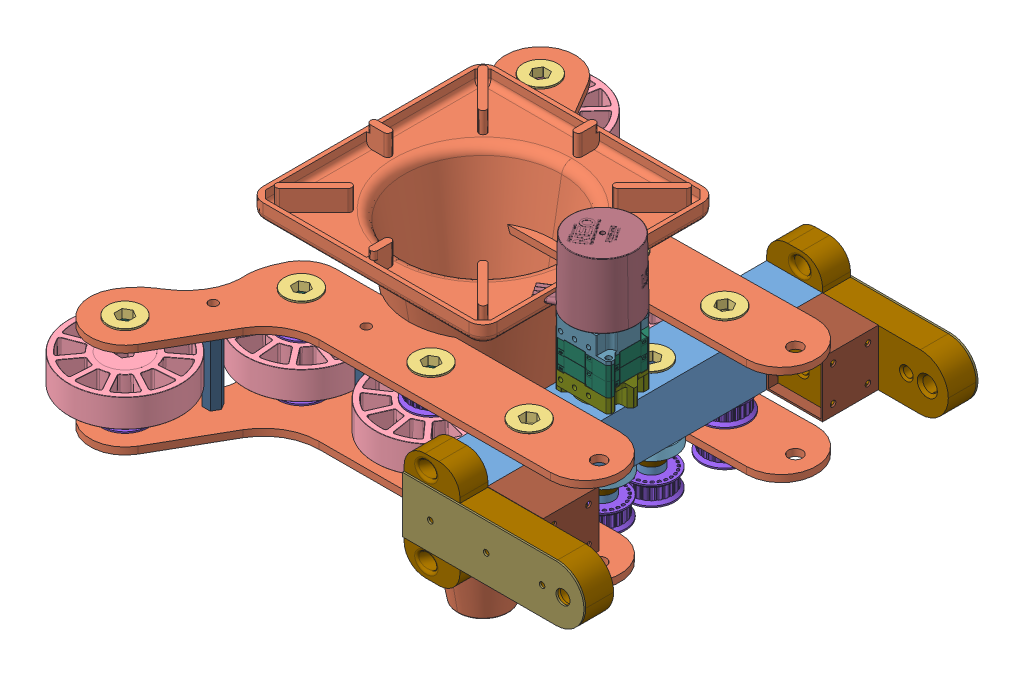
SolidWorks assembly Intake_Claw_2.0, configuration Default. Lengths in mm.
Overall size (474.27 365.54 510.07).
111 component instances, 20 part files, 307 mates.
Components (placement in the parent):
- Claw_Crossbar-1: Claw_Crossbar [Default] at origin size (50.8 50.8 304.8)
- Claw_Intake_Plate_3_Wheel-3: Claw_Intake_Plate_3_Wheel [Default] at (-63.4996 52.3773 241.5528) x (-0.002844 0 -0.999996) z (0.999996 0 -0.002844) size (165.24 6.35 379.41)
- am-2986 FR8ZZ Hex Bearing.step-1: am-2986 FR8ZZ Hex Bearing.step [Default] at (25.4 44.3967 241.3) x (-0.023449 0 -0.999725) z (0 1 0) size (31.12 31.12 7.93)
- am-2986 FR8ZZ Hex Bearing.step-3: am-2986 FR8ZZ Hex Bearing.step [Default] at (-239.4221 52.324 343.7898) x (0 0 -1) z (0 1 0) size (31.12 31.12 7.93)
- am-2986 FR8ZZ Hex Bearing.step-5: am-2986 FR8ZZ Hex Bearing.step [Default] at (25.4 52.324 241.3) x (0 0 -1) z (0 1 0) size (31.12 31.12 7.93)
- am-2986 FR8ZZ Hex Bearing.step-11: am-2986 FR8ZZ Hex Bearing.step [Default] at (-63.4996 52.324 241.5528) x (0 0 -1) z (0 1 0) size (31.12 31.12 7.93)
- am-2986 FR8ZZ Hex Bearing.step-12: am-2986 FR8ZZ Hex Bearing.step [Default] at (-180.9742 52.324 241.8869) x (0 0 -1) z (0 1 0) size (31.12 31.12 7.93)
- Intake_Plate_Assembly-1: Intake_Plate_Assembly [Default] at (-25.3851 110.6877 261.8842) x (0.99204 0 0.125922) z (0.125922 0 -0.99204)
- Intake_Plate_Assembly_2-1: Intake_Plate_Assembly_2 [Default] at (-16.4979 -120.1924 40.8533) x (0.996656 0 -0.081713) z (0.081713 0 0.996656)
- Intake_Plate_Assembly_2-2: Intake_Plate_Assembly_2 [Default] at (-25.364 170.9924 261.8868) x (0.99204 0 0.125922) z (0.125922 0 -0.99204)
- am-3480 4IN 500Hex Bore Compliant Wheel REV2.STEP-1: am-3480 4IN 500Hex Bore Compliant Wheel REV2.STEP [Default] at (-227.1156 24.621 332.519) x (0.873407 0 -0.486991) z (0 -1 0) size (101.6 101.6 25.4)
- am-3480 4IN 500Hex Bore Compliant Wheel REV2.STEP-2: am-3480 4IN 500Hex Bore Compliant Wheel REV2.STEP [Default] at (-170.4614 24.621 228.9267) x (0.792175 0 -0.610293) z (0 -1 0) size (101.6 101.6 25.4)
- am-3480 4IN 500Hex Bore Compliant Wheel REV2.STEP-3: am-3480 4IN 500Hex Bore Compliant Wheel REV2.STEP [Default] at (-68.8044 24.621 257.3751) x (-0.528092 0 0.849187) z (0 -1 0) size (101.6 101.6 25.4)
- am-3480 4IN 500Hex Bore Compliant Wheel REV2.STEP-4: am-3480 4IN 500Hex Bore Compliant Wheel REV2.STEP [Default] at (-47.059 24.621 61.63) x (0.998282 0 0.058584) z (0 -1 0) size (101.6 101.6 25.4)
- am-3480 4IN 500Hex Bore Compliant Wheel REV2.STEP-5: am-3480 4IN 500Hex Bore Compliant Wheel REV2.STEP [Default] at (-164.7239 24.621 62.024) x (1 0 0) z (0 -1 0) size (101.6 101.6 25.4)
- am-3480 4IN 500Hex Bore Compliant Wheel REV2.STEP-6: am-3480 4IN 500Hex Bore Compliant Wheel REV2.STEP [Default] at (-248.6981 24.621 -49.9144) x (-0.252916 0 -0.967488) z (0 -1 0) size (101.6 101.6 25.4)
- am-2986 FR8ZZ Hex Bearing.step-13: am-2986 FR8ZZ Hex Bearing.step [Default] at (25.4 6.4033 130.175) x (-0.368447 0 0.929649) z (0 -1 0) size (31.12 31.12 7.93)
- am-2986 FR8ZZ Hex Bearing.step-14: am-2986 FR8ZZ Hex Bearing.step [Default] at (25.4 44.3967 130.175) x (-0.368447 0 0.929649) z (0 1 0) size (31.12 31.12 7.93)
- Claw_Drive_Gear-1: Claw_Drive_Gear [Default] at (25.4 -14.1478 130.175) x (0.993752 0 0.111608) z (-0.111608 0 0.993752) size (43.69 9.45 43.69)
- Claw_Drive_Gear-2: Claw_Drive_Gear [Default] at (25.4 -14.1478 174.625) x (0.964298 0 0.26482) z (-0.26482 0 0.964298) size (43.69 9.45 43.69)
- half_inch_hex_spacer_0.125inch-1: half_inch_hex_spacer_0.125inch [Default] at (25.4 -4.699 130.175) x (0.999916 0 -0.012929) z (0.012929 0 0.999916) size (20.32 3.17 20.32)
- half_inch_hex_spacer_0.125inch-2: half_inch_hex_spacer_0.125inch [Default] at (25.4 -4.699 174.625) x (0.980488 0 0.196577) z (-0.196577 0 0.980488) size (20.32 3.17 20.32)
- am-2986 FR8ZZ Hex Bearing.step-16: am-2986 FR8ZZ Hex Bearing.step [Default] at (25.4 44.3967 63.5) x (-0.023449 0 -0.999725) z (0 1 0) size (31.12 31.12 7.93)
- am-2986 FR8ZZ Hex Bearing.step-18: am-2986 FR8ZZ Hex Bearing.step [Default] at (25.4 6.4033 63.5) x (-0.368447 0 0.929649) z (0 -1 0) size (31.12 31.12 7.93)
- am-2986 FR8ZZ Hex Bearing.step-19: am-2986 FR8ZZ Hex Bearing.step [Default] at (25.4 6.4033 241.3) x (-0.368447 0 0.929649) z (0 -1 0) size (31.12 31.12 7.93)
- half_inch_hex_spacer_0.1875inch-1: half_inch_hex_spacer_0.1875inch [Default] at (25.4 52.324 63.5) size (20.32 4.76 20.32)
- 24_tooth_5mmHTD_timing_belt_pulley_9mm-3: 24_tooth_5mmHTD_timing_belt_pulley_9mm [Default] at (-180.9742 35.179 241.8869) x (0.987086 0 0.160191) z (0 -1 0) size (42.16 42.16 17.78)
- 24_tooth_5mmHTD_timing_belt_pulley_9mm-8: 24_tooth_5mmHTD_timing_belt_pulley_9mm [Default] at (25.4 -47.1678 174.625) x (0.071014 0 0.997475) z (0 -1 0) size (42.16 42.16 17.78)
- 24_tooth_5mmHTD_timing_belt_pulley_9mm-9: 24_tooth_5mmHTD_timing_belt_pulley_9mm [Default] at (25.4 -47.1678 130.175) x (0.476247 0 -0.879312) z (0 -1 0) size (42.16 42.16 17.78)
- 24_tooth_5mmHTD_timing_belt_pulley_9mm-13: 24_tooth_5mmHTD_timing_belt_pulley_9mm [Default] at (-180.9613 35.179 65.8749) x (0.911482 0 -0.411341) z (0 -1 0) size (42.16 42.16 17.78)
- 24_tooth_5mmHTD_timing_belt_pulley_9mm-15: 24_tooth_5mmHTD_timing_belt_pulley_9mm [Default] at (-63.4996 35.179 241.5528) x (0.911482 0 -0.411341) z (0 -1 0) size (42.16 42.16 17.78)
- 24_tooth_5mmHTD_timing_belt_pulley_9mm-16: 24_tooth_5mmHTD_timing_belt_pulley_9mm [Default] at (-63.4941 35.179 64.523) x (0.84545 0 -0.534054) z (0 -1 0) size (42.16 42.16 17.78)
- half_inch_hex_spacer_0.125inch-13: half_inch_hex_spacer_0.125inch [Default] at (-63.4941 2.794 64.523) size (20.32 3.17 20.32)
- half_inch_hex_spacer_0.125inch-14: half_inch_hex_spacer_0.125inch [Default] at (-180.9613 2.794 65.8749) size (20.32 3.17 20.32)
- half_inch_hex_spacer_0.125inch-15: half_inch_hex_spacer_0.125inch [Default] at (-240.8657 2.794 -35.1788) size (20.32 3.17 20.32)
- half_inch_hex_spacer_0.125inch-16: half_inch_hex_spacer_0.125inch [Default] at (-63.4996 2.794 241.5528) size (20.32 3.17 20.32)
- half_inch_hex_spacer_0.125inch-17: half_inch_hex_spacer_0.125inch [Default] at (-180.9742 2.794 241.8869) size (20.32 3.17 20.32)
- half_inch_hex_spacer_0.125inch-18: half_inch_hex_spacer_0.125inch [Default] at (-239.4221 2.794 343.7898) size (20.32 3.17 20.32)
- Grabber_Spring_Mount-1: Grabber_Spring_Mount [Default] at (49.2125 48.5775 260.35) x (-1 0 0) z (0 0 1) size (165.1 97.79 69.85)
- Grabber_Spring_Mount-2: Grabber_Spring_Mount [Default] at (48.5775 1.5875 44.45) x (-1 0 0) z (0 0 -1) size (165.1 97.79 69.85)
- 24_tooth_5mmHTD_timing_belt_pulley_9mm-17: 24_tooth_5mmHTD_timing_belt_pulley_9mm [Default] at (25.4 -18.669 241.3) x (0.782455 0 -0.622708) z (0 -1 0) size (42.16 42.16 17.78)
- 24_tooth_5mmHTD_timing_belt_pulley_9mm-18: 24_tooth_5mmHTD_timing_belt_pulley_9mm [Default] at (25.4 -18.669 63.5) x (0.782455 0 -0.622708) z (0 -1 0) size (42.16 42.16 17.78)
- half_inch_hex_spacer_0.125inch-19: half_inch_hex_spacer_0.125inch [Default] at (25.4 -4.699 63.5) size (20.32 3.17 20.32)
- half_inch_hex_spacer_0.125inch-20: half_inch_hex_spacer_0.125inch [Default] at (25.4 -4.699 241.3) size (20.32 3.17 20.32)
- half_inch_hex_spacer_0.125inch-21: half_inch_hex_spacer_0.125inch [Default] at (-63.4941 -0.381 64.523) size (20.32 3.17 20.32)
- half_inch_hex_spacer_0.125inch-22: half_inch_hex_spacer_0.125inch [Default] at (-180.9613 -0.381 65.8749) size (20.32 3.17 20.32)
- half_inch_hex_spacer_0.125inch-23: half_inch_hex_spacer_0.125inch [Default] at (-240.8657 -0.381 -35.1788) size (20.32 3.17 20.32)
- half_inch_hex_spacer_0.125inch-24: half_inch_hex_spacer_0.125inch [Default] at (-239.4221 -0.381 343.7898) size (20.32 3.17 20.32)
- half_inch_hex_spacer_0.125inch-25: half_inch_hex_spacer_0.125inch [Default] at (-180.9742 -0.381 241.8869) size (20.32 3.17 20.32)
- half_inch_hex_spacer_0.125inch-26: half_inch_hex_spacer_0.125inch [Default] at (-63.4996 -0.381 241.5528) size (20.32 3.17 20.32)
- half_inch_hex_spacer_0.125inch-27: half_inch_hex_spacer_0.125inch [Default] at (-63.4996 -21.336 241.5528) size (20.32 3.17 20.32)
- half_inch_hex_spacer_0.125inch-28: half_inch_hex_spacer_0.125inch [Default] at (-180.9742 -21.336 241.8869) size (20.32 3.17 20.32)
- half_inch_hex_spacer_0.125inch-29: half_inch_hex_spacer_0.125inch [Default] at (-239.4221 -21.336 343.7898) size (20.32 3.17 20.32)
- half_inch_hex_spacer_0.125inch-30: half_inch_hex_spacer_0.125inch [Default] at (-63.4941 -21.336 64.523) size (20.32 3.17 20.32)
- half_inch_hex_spacer_0.125inch-31: half_inch_hex_spacer_0.125inch [Default] at (-180.9613 -21.336 65.8749) size (20.32 3.17 20.32)
- half_inch_hex_spacer_0.125inch-32: half_inch_hex_spacer_0.125inch [Default] at (-240.8657 -21.336 -35.1788) size (20.32 3.17 20.32)
- 24_tooth_5mmHTD_timing_belt_pulley_9mm-19: 24_tooth_5mmHTD_timing_belt_pulley_9mm [Default] at (-63.4941 -14.351 64.523) x (1 0 0) z (0 -1 0) size (42.16 42.16 17.78)
- 24_tooth_5mmHTD_timing_belt_pulley_9mm-20: 24_tooth_5mmHTD_timing_belt_pulley_9mm [Default] at (-180.9613 -14.351 65.8749) x (1 0 0) z (0 -1 0) size (42.16 42.16 17.78)
- 24_tooth_5mmHTD_timing_belt_pulley_9mm-21: 24_tooth_5mmHTD_timing_belt_pulley_9mm [Default] at (-240.8657 -14.351 -35.1788) x (1 0 0) z (0 -1 0) size (42.16 42.16 17.78)
- 24_tooth_5mmHTD_timing_belt_pulley_9mm-22: 24_tooth_5mmHTD_timing_belt_pulley_9mm [Default] at (-239.4221 -14.351 343.7898) x (1 0 0) z (0 -1 0) size (42.16 42.16 17.78)
- 24_tooth_5mmHTD_timing_belt_pulley_9mm-23: 24_tooth_5mmHTD_timing_belt_pulley_9mm [Default] at (-180.9742 -14.351 241.8869) x (1 0 0) z (0 -1 0) size (42.16 42.16 17.78)
- 24_tooth_5mmHTD_timing_belt_pulley_9mm-24: 24_tooth_5mmHTD_timing_belt_pulley_9mm [Default] at (-63.4996 -14.351 241.5528) x (1 0 0) z (0 -1 0) size (42.16 42.16 17.78)
- half_inch_hex_spacer_0.125inch-33: half_inch_hex_spacer_0.125inch [Default] at (25.4 -25.654 63.5) size (20.32 3.17 20.32)
- half_inch_hex_spacer_0.125inch-34: half_inch_hex_spacer_0.125inch [Default] at (25.4 -25.654 241.3) size (20.32 3.17 20.32)
- Intake_Plate_Assembly-3: Intake_Plate_Assembly [Default] at (-25.3851 78.6304 261.8842) x (0.99204 0 0.125922) z (0.125922 0 -0.99204)
- Intake_Plate_Assembly_2-4: Intake_Plate_Assembly_2 [Default] at (-16.4979 -152.2498 40.8533) x (0.996656 0 -0.081713) z (0.081713 0 0.996656)
- grabber_stand_off-1: grabber_stand_off [Default] at (-122.2369 52.3977 241.7198) x (1 0 0) z (0 -1 0) size (14.66 12.7 76.2)
- grabber_stand_off-3: grabber_stand_off [Default] at (-210.1981 52.3773 292.8384) x (1 0 0) z (0 -1 0) size (14.66 12.7 76.2)
- grabber_stand_off-4: grabber_stand_off [Default] at (-210.9135 44.5398 15.3481) x (-0.606361 0 0.795189) z (0 -1 0) size (14.66 12.7 76.2)
- grabber_stand_off-5: grabber_stand_off [Default] at (-122.2277 50.6322 65.199) x (1 0 0) z (0 -1 0) size (14.66 12.7 76.2)
- Crossbar_Bracket-1: Crossbar_Bracket [Default] at (101.6 0 0) x (0 1 0) z (0 0 1) size (50.8 50.8 50.8)
- Crossbar_Bracket-2: Crossbar_Bracket [Default] at (101.6 0 254) x (0 1 0) z (0 0 1) size (50.8 50.8 50.8)
- Claw_Pivot_Plate-1: Claw_Pivot_Plate [Default] at (0.635 -0.3175 330.2) size (165.1 50.8 1.59)
- Claw_Pivot_Plate-2: Claw_Pivot_Plate [Default] at (0 -0.3175 -26.9875) size (165.1 50.8 1.59)
- half_inch_hex_spacer_0.125inch-35: half_inch_hex_spacer_0.125inch [Default] at (-63.4996 49.149 241.5528) size (20.32 3.17 20.32)
- half_inch_hex_spacer_0.125inch-36: half_inch_hex_spacer_0.125inch [Default] at (-180.9742 49.149 241.8869) size (20.32 3.17 20.32)
- half_inch_hex_spacer_0.125inch-37: half_inch_hex_spacer_0.125inch [Default] at (-239.4221 49.149 343.7898) size (20.32 3.17 20.32)
- half_inch_hex_spacer_0.125inch-38: half_inch_hex_spacer_0.125inch [Default] at (-63.4941 49.149 64.523) size (20.32 3.17 20.32)
- half_inch_hex_spacer_0.125inch-39: half_inch_hex_spacer_0.125inch [Default] at (-180.9613 49.149 65.8749) size (20.32 3.17 20.32)
- Claw_Intake_Plate_3_Wheel-4: Claw_Intake_Plate_3_Wheel [Default] at (-63.4996 -27.7393 241.5528) x (-0.002844 0 -0.999996) z (0.999996 0 -0.002844) size (165.24 6.35 379.41)
- Claw_Intake_Plate_3_Wheel-5: Claw_Intake_Plate_3_Wheel [Default] at (-63.4941 58.7273 64.523) x (0.011508 0 0.999934) z (0.999934 0 -0.011508) size (165.24 6.35 379.41)
- Claw_Intake_Plate_3_Wheel-6: Claw_Intake_Plate_3_Wheel [Default] at (-63.4941 -25.7073 64.523) x (0.011508 0 0.999934) z (0.999934 0 -0.011508) size (165.24 6.35 379.41)
- am-2986 FR8ZZ Hex Bearing.step-20: am-2986 FR8ZZ Hex Bearing.step [Default] at (25.4 -21.336 241.3) x (1 0 0) z (0 -1 0) size (31.12 31.12 7.93)
- am-2986 FR8ZZ Hex Bearing.step-21: am-2986 FR8ZZ Hex Bearing.step [Default] at (-63.4996 -21.336 241.5528) x (0.820291 0 -0.571946) z (0 -1 0) size (31.12 31.12 7.93)
- am-2986 FR8ZZ Hex Bearing.step-22: am-2986 FR8ZZ Hex Bearing.step [Default] at (-180.9742 -21.336 241.8869) x (1 0 0) z (0 -1 0) size (31.12 31.12 7.93)
- am-2986 FR8ZZ Hex Bearing.step-23: am-2986 FR8ZZ Hex Bearing.step [Default] at (-239.4221 -21.336 343.7898) x (1 0 0) z (0 -1 0) size (31.12 31.12 7.93)
- am-2986 FR8ZZ Hex Bearing.step-24: am-2986 FR8ZZ Hex Bearing.step [Default] at (25.4 -25.654 63.5) x (1 0 0) z (0 -1 0) size (31.12 31.12 7.93)
- am-2986 FR8ZZ Hex Bearing.step-25: am-2986 FR8ZZ Hex Bearing.step [Default] at (-63.4941 -25.654 64.523) x (1 0 0) z (0 -1 0) size (31.12 31.12 7.93)
- am-2986 FR8ZZ Hex Bearing.step-26: am-2986 FR8ZZ Hex Bearing.step [Default] at (-240.8657 -25.654 -35.1788) x (1 0 0) z (0 -1 0) size (31.12 31.12 7.93)
- am-2986 FR8ZZ Hex Bearing.step-27: am-2986 FR8ZZ Hex Bearing.step [Default] at (-180.9613 -25.654 65.8749) x (1 0 0) z (0 -1 0) size (31.12 31.12 7.93)
- am-2986 FR8ZZ Hex Bearing.step-28: am-2986 FR8ZZ Hex Bearing.step [Default] at (25.4 52.324 63.5) x (1 0 0) z (0 1 0) size (31.12 31.12 7.93)
- am-2986 FR8ZZ Hex Bearing.step-29: am-2986 FR8ZZ Hex Bearing.step [Default] at (-63.4941 52.324 64.523) x (1 0 0) z (0 1 0) size (31.12 31.12 7.93)
- am-2986 FR8ZZ Hex Bearing.step-30: am-2986 FR8ZZ Hex Bearing.step [Default] at (-180.9613 52.324 65.8749) x (1 0 0) z (0 1 0) size (31.12 31.12 7.93)
- am-2986 FR8ZZ Hex Bearing.step-31: am-2986 FR8ZZ Hex Bearing.step [Default] at (-240.8657 52.324 -35.1788) x (1 0 0) z (0 1 0) size (31.12 31.12 7.93)
- am-2986 FR8ZZ Hex Bearing.step-32: am-2986 FR8ZZ Hex Bearing.step [Default] at (25.4 6.4033 174.625) x (-0.500268 0 0.865871) z (0 -1 0) size (31.12 31.12 7.93)
- Neo_with_2_Stage_Gearbox-1: Neo_with_2_Stage_Gearbox [Default] at (26.2874 219.325 175.8085) x (0.980561 0 0.196216) z (0 -1 0) size (73.48 69 161.54)
  - REV-21-1650-V1.1.step-1: REV-21-1650-V1.1.step [Default] at (-1.1023 -0.9864 105.025) size (68.13 68.01 93.35)
  - REV-21-2106.step-1: REV-21-2106.step [Default] at (-1.1023 -0.9864 114.55) x (0.980561 -0.196216 0) z (0 0 1) size (61.91 50.8 19.05)
  - REV-21-2103.step-1: REV-21-2103.step [Default] at (-1.1023 -0.9864 130.425) x (0.980561 -0.196216 0) z (0 0 1) size (61.91 50.8 16.85)
  - REV-21-2104.step-1: REV-21-2104.step [Default] at (-1.1023 -0.9864 159) x (0 0 1) z (-0.980561 0.196216 0) size (23.2 50.8 61.92)
  - REV-21-2103.step-2: REV-21-2103.step [Default] at (-1.1023 -0.9864 143.125) x (0.980561 -0.196216 0) z (0 0 1) size (61.91 50.8 16.85)
  - motor_drive_shaft-1: motor_drive_shaft [Default] at (-1.1023 -0.9864 157.4125) x (0.217469 0.976067 0) z (0 0 1) size (14.66 12.7 50.8)
- half_inch_hex_spacer_0.125inch-40: half_inch_hex_spacer_0.125inch [Default] at (25.4 -36.7563 63.5) x (0.980488 0 0.196577) z (-0.196577 0 0.980488) size (20.32 3.17 20.32)
- half_inch_hex_spacer_0.125inch-41: half_inch_hex_spacer_0.125inch [Default] at (25.4 -32.4383 241.3) x (0.980488 0 0.196577) z (-0.196577 0 0.980488) size (20.32 3.17 20.32)
- 24_tooth_5mmHTD_timing_belt_pulley_9mm-25: 24_tooth_5mmHTD_timing_belt_pulley_9mm [Default] at (25.4 -50.7263 63.5) x (1 0 0) z (0 -1 0) size (42.16 42.16 17.78)
- 24_tooth_5mmHTD_timing_belt_pulley_9mm-26: 24_tooth_5mmHTD_timing_belt_pulley_9mm [Default] at (25.4 -46.4083 241.3) x (1 0 0) z (0 -1 0) size (42.16 42.16 17.78)
- half_inch_hex_spacer_0.5inch-1: half_inch_hex_spacer_0.5inch [Default] at (25.4 -26.8478 130.175) size (20.32 12.7 20.32)
- half_inch_hex_spacer_0.5inch-2: half_inch_hex_spacer_0.5inch [Default] at (25.4 -26.8478 174.625) size (20.32 12.7 20.32)
- half_inch_hex_spacer_0.25inch-1: half_inch_hex_spacer_0.25inch [Default] at (25.4 -33.1978 130.175) size (20.32 6.35 20.32)
- half_inch_hex_spacer_0.25inch-2: half_inch_hex_spacer_0.25inch [Default] at (25.4 -33.1978 174.625) size (20.32 6.35 20.32)
- am-4700_syc Cone-1: am-4700_syc Cone [Default] at (-106.3625 125.4023 151.5086) x (1 0 0) z (0 0 -1) size (212.72 325.44 212.72)
Mates (geometry in assembly coordinates):
- Concentric2: concentric aligned: circle of Claw_Crossbar-1; circle of Claw_Intake_Plates-3
- Concentric5: concentric aligned: circle of Claw_Crossbar-1; circle of am-2986 FR8ZZ Hex Bearing.step-1
- Coincident11: coincident anti-aligned: plane of Claw_Crossbar-1 through (0 50.8 304.8) normal (0 1 0); plane of am-2986 FR8ZZ Hex Bearing.step-1 through (25.0724 50.8 227.3338) normal (0 -1 0)
- Concentric6: concentric anti-aligned: cylinder of Claw_Intake_Plates-3; cylinder of am-2986 FR8ZZ Hex Bearing.step-5 through (25.4 60.2513 241.3) axis (0 -1 0) radius 15.5575
- Coincident12: coincident anti-aligned: plane of Claw_Intake_Plates-3 through (-239.4221 58.7273 343.7898) normal (0 1 0); plane of am-2986 FR8ZZ Hex Bearing.step-5 through (25.4 58.7273 227.33) normal (0 -1 0)
- Concentric7: concentric aligned: circle of Claw_Intake_Plates-3; circle of am-2986 FR8ZZ Hex Bearing.step-11
- Coincident13: coincident anti-aligned: plane of Claw_Intake_Plates-3 through (-239.4221 58.7273 343.7898) normal (0 1 0); plane of am-2986 FR8ZZ Hex Bearing.step-11 through (-63.4996 58.7273 227.5828) normal (0 -1 0)
- Concentric8: concentric aligned: circle of Claw_Intake_Plates-3; circle of am-2986 FR8ZZ Hex Bearing.step-12
- Coincident14: coincident anti-aligned: plane of Claw_Intake_Plates-3 through (-239.4221 58.7273 343.7898) normal (0 1 0); plane of am-2986 FR8ZZ Hex Bearing.step-12 through (-180.9742 58.7273 227.9169) normal (0 -1 0)
- Concentric9: concentric aligned: circle of Claw_Intake_Plates-3; circle of am-2986 FR8ZZ Hex Bearing.step-3
- Coincident15: coincident anti-aligned: plane of Claw_Intake_Plates-3 through (-239.4221 58.7273 343.7898) normal (0 1 0); plane of am-2986 FR8ZZ Hex Bearing.step-3 through (-239.4221 58.7273 329.8198) normal (0 -1 0)
- Concentric10: concentric anti-aligned: circle of Claw_Crossbar-1; circle of Intake_Plate_Assembly-1/am-2986 FR8ZZ Hex Bearing.step-5
- Concentric11: concentric aligned: circle of Claw_Crossbar-1; circle of Intake_Plate_Assembly_2-1/Claw_Intake_Plates-3
- Concentric12: concentric anti-aligned: circle of Claw_Crossbar-1; circle of Intake_Plate_Assembly_2-2/Claw_Intake_Plates-3
- Parallel3: parallel aligned: plane of Intake_Plate_Assembly-1/Claw_Intake_Plates-3 through (77.0074 -7.9273 33.08) normal (0.025971 0 -0.999663); plane of Intake_Plate_Assembly_2-2/Claw_Intake_Plates-3 through (77.0074 52.3773 33.08) normal (0.025971 0 -0.999663)
- Parallel4: parallel aligned: plane of Claw_Intake_Plates-3 through (76.2901 58.7273 272.9054) normal (0.002844 0 0.999996); plane of Intake_Plate_Assembly_2-1/Claw_Intake_Plates-3 through (75.6047 -1.5773 273.9833) normal (-0.018478 0 0.999829)
- Concentric17: concentric anti-aligned: circle of Intake_Plate_Assembly_2-1/am-2986 FR8ZZ Hex Bearing.step-18; circle of am-3480 4IN 500Hex Bore Compliant Wheel REV2.STEP-1
- Concentric18: concentric anti-aligned: circle of Intake_Plate_Assembly_2-1/am-2986 FR8ZZ Hex Bearing.step-17; circle of am-3480 4IN 500Hex Bore Compliant Wheel REV2.STEP-2
- Concentric20: concentric anti-aligned: circle of Intake_Plate_Assembly-1/am-2986 FR8ZZ Hex Bearing.step-12; circle of am-3480 4IN 500Hex Bore Compliant Wheel REV2.STEP-5
- Concentric21: concentric aligned: circle of Intake_Plate_Assembly-1/am-2986 FR8ZZ Hex Bearing.step-11; circle of am-3480 4IN 500Hex Bore Compliant Wheel REV2.STEP-4
- Concentric22: concentric anti-aligned: circle of Intake_Plate_Assembly-1/am-2986 FR8ZZ Hex Bearing.step-3; circle of am-3480 4IN 500Hex Bore Compliant Wheel REV2.STEP-6
- Coincident21: coincident aligned: plane of am-3480 4IN 500Hex Bore Compliant Wheel REV2.STEP-5 through (-180.9613 5.969 86.3864) normal (0 -1 0); plane of am-3480 4IN 500Hex Bore Compliant Wheel REV2.STEP-6 through (-221.0211 5.969 -40.3665) normal (0 -1 0)
- Coincident22: coincident aligned: plane of am-3480 4IN 500Hex Bore Compliant Wheel REV2.STEP-4 through (-64.6958 5.969 84.9993) normal (0 -1 0); plane of am-3480 4IN 500Hex Bore Compliant Wheel REV2.STEP-5 through (-180.9613 5.969 86.3864) normal (0 -1 0)
- Coincident23: coincident aligned: plane of am-3480 4IN 500Hex Bore Compliant Wheel REV2.STEP-2 through (-168.4561 5.969 258.1356) normal (0 -1 0); plane of am-3480 4IN 500Hex Bore Compliant Wheel REV2.STEP-4 through (-64.6958 5.969 84.9993) normal (0 -1 0)
- Coincident24: coincident aligned: plane of am-3480 4IN 500Hex Bore Compliant Wheel REV2.STEP-1 through (-229.4332 5.969 361.7047) normal (0 -1 0); plane of am-3480 4IN 500Hex Bore Compliant Wheel REV2.STEP-2 through (-168.4561 5.969 258.1356) normal (0 -1 0)
- Coincident25: coincident aligned: plane of am-3480 4IN 500Hex Bore Compliant Wheel REV2.STEP-1 through (-229.4332 5.969 361.7047) normal (0 -1 0); plane of am-3480 4IN 500Hex Bore Compliant Wheel REV2.STEP-3 through (-80.9178 5.969 230.7209) normal (0 -1 0)
- Concentric23: concentric anti-aligned: circle of Intake_Plate_Assembly_2-1/am-2986 FR8ZZ Hex Bearing.step-11; circle of am-3480 4IN 500Hex Bore Compliant Wheel REV2.STEP-3
- Coincident26: coincident aligned: plane of Intake_Plate_Assembly-1/Claw_Intake_Plates-3 through (-236.9809 -7.9273 -45.0872) normal (0 -1 0); plane of Intake_Plate_Assembly_2-1/Claw_Intake_Plates-3 through (-241.5471 -7.9273 338.1202) normal (0 -1 0)
- Coincident27: coincident aligned: plane of Claw_Intake_Plates-3 through (-239.4221 52.3773 343.7898) normal (0 -1 0); plane of Intake_Plate_Assembly_2-2/Claw_Intake_Plates-3 through (-236.9809 52.3773 -45.0872) normal (0 -1 0)
- Parallel6: parallel aligned: plane of Claw_Crossbar-1 through (50.8 0 304.8) normal (1 0 0); plane of REV-21-2103.step-1 through (50.8 -18.7019 200.025) normal (1 0 0)
- Concentric26: concentric anti-aligned: circle of Claw_Crossbar-1; circle of am-2986 FR8ZZ Hex Bearing.step-13
- Coincident30: coincident anti-aligned: plane of Claw_Crossbar-1 through (0 0 304.8) normal (0 -1 0); plane of am-2986 FR8ZZ Hex Bearing.step-13 through (20.2528 0 143.1622) normal (0 1 0)
- Concentric27: concentric anti-aligned: circle of Claw_Crossbar-1; circle of am-2986 FR8ZZ Hex Bearing.step-14
- Concentric28: concentric anti-aligned: circle of Claw_Crossbar-1; circle of am-2986 FR8ZZ Hex Bearing.step-15
- Coincident31: coincident anti-aligned: plane of Claw_Crossbar-1 through (0 50.8 304.8) normal (0 1 0); plane of am-2986 FR8ZZ Hex Bearing.step-15 through (20.2528 50.8 187.6122) normal (0 -1 0)
- Coincident32: coincident anti-aligned: plane of Claw_Crossbar-1 through (0 50.8 304.8) normal (0 1 0); plane of am-2986 FR8ZZ Hex Bearing.step-14 through (20.2528 50.8 143.1622) normal (0 -1 0)
- Concentric29: concentric aligned: circle of am-2986 FR8ZZ Hex Bearing.step-14; circle of Claw_Drive_Gear-1
- Concentric30: concentric anti-aligned: circle of am-2986 FR8ZZ Hex Bearing.step-15; circle of Claw_Drive_Gear-2
- Concentric31: concentric anti-aligned: circle of am-2986 FR8ZZ Hex Bearing.step-14; circle of half_inch_hex_spacer_0.125inch-1
- Concentric32: concentric anti-aligned: circle of am-2986 FR8ZZ Hex Bearing.step-15; circle of half_inch_hex_spacer_0.125inch-2
- Coincident37: coincident anti-aligned: plane of Claw_Drive_Gear-1 through (25.4 -4.699 130.175) normal (0 1 0); plane of half_inch_hex_spacer_0.125inch-3 through (25.4 64.9478 130.556) normal (0 -1 0)
- Concentric33: concentric aligned: circle of Claw_Drive_Gear-1; circle of half_inch_hex_spacer_0.125inch-3
- Coincident38: coincident anti-aligned: plane of Claw_Drive_Gear-2 through (25.4 -4.699 174.625) normal (0 1 0); plane of half_inch_hex_spacer_0.125inch-4 through (25.4 64.9478 174.244) normal (0 -1 0)
- Concentric34: concentric aligned: circle of Claw_Drive_Gear-2; circle of half_inch_hex_spacer_0.125inch-4
- Coincident39: coincident anti-aligned: plane of Claw_Crossbar-1 through (0 50.8 304.8) normal (0 1 0); plane of am-2986 FR8ZZ Hex Bearing.step-16 through (25.0724 50.8 49.5338) normal (0 -1 0)
- Concentric35: concentric anti-aligned: circle of Claw_Crossbar-1; circle of am-2986 FR8ZZ Hex Bearing.step-16
- Coincident40: coincident anti-aligned: plane of Claw_Crossbar-1 through (0 0 304.8) normal (0 -1 0); plane of am-2986 FR8ZZ Hex Bearing.step-18 through (20.2528 0 76.4872) normal (0 1 0)
- Coincident41: coincident anti-aligned: plane of Claw_Crossbar-1 through (0 0 304.8) normal (0 -1 0); plane of am-2986 FR8ZZ Hex Bearing.step-19 through (20.2528 0 254.2872) normal (0 1 0)
- Concentric36: concentric anti-aligned: circle of Claw_Crossbar-1; circle of am-2986 FR8ZZ Hex Bearing.step-19
- Concentric37: concentric anti-aligned: circle of Claw_Crossbar-1; circle of am-2986 FR8ZZ Hex Bearing.step-18
- Coincident42: coincident anti-aligned: plane of Intake_Plate_Assembly_2-1/am-2986 FR8ZZ Hex Bearing.step-16 through (25.4 -1.524 241.3) normal (0 1 0); plane of am-2986 FR8ZZ Hex Bearing.step-19 through (19.6679 -1.524 255.763) normal (0 -1 0)
- Coincident43: coincident anti-aligned: plane of am-2986 FR8ZZ Hex Bearing.step-1 through (25.0352 52.324 225.7468) normal (0 1 0); plane of am-2986 FR8ZZ Hex Bearing.step-5 through (25.4 52.324 241.3) normal (0 -1 0)
- Coincident45: coincident anti-aligned: plane of Claw_Drive_Gear-1 through (25.4 -4.699 130.175) normal (0 1 0); plane of 18_tooth_5mmHTD_timing_belt_pulley_9mm-1 through (25.4 64.9478 130.556) normal (0 -1 0)
- Concentric39: concentric aligned: circle of Claw_Drive_Gear-1; circle of 18_tooth_5mmHTD_timing_belt_pulley_9mm-1
- Parallel7: parallel anti-aligned: plane of Claw_Drive_Gear-2 through (25.4 -14.1478 174.625) normal (0 -1 0); plane of half_inch_hex_spacer_0.125inch-4 through (25.4 68.1228 174.244) normal (0 1 0)
- Coincident48: coincident anti-aligned: plane of 18_tooth_5mmHTD_timing_belt_pulley_9mm-1 through (25.4 82.7278 130.556) normal (0 1 0); plane of half_inch_hex_collar-2 through (25.4 82.7278 130.556) normal (0 -1 0)
- Concentric42: concentric aligned: circle of 18_tooth_5mmHTD_timing_belt_pulley_9mm-1; circle of half_inch_hex_collar-2
- Coincident50: coincident anti-aligned: plane of am-2986 FR8ZZ Hex Bearing.step-5 through (25.4 60.2513 225.7425) normal (0 1 0); plane of half_inch_hex_spacer_0.125inch-5 through (25.4 60.2513 241.3) normal (0 -1 0)
- Coincident51: coincident aligned: plane of Intake_Plate_Assembly_2-2/am-2986 FR8ZZ Hex Bearing.step-16 through (23.441 60.2513 78.9337) normal (0 1 0); circle of half_inch_hex_spacer_0.125inch-6
- Concentric43: concentric aligned: circle of Intake_Plate_Assembly_2-2/am-2986 FR8ZZ Hex Bearing.step-16; circle of half_inch_hex_spacer_0.125inch-6
- Concentric44: concentric aligned: circle of am-2986 FR8ZZ Hex Bearing.step-5; circle of half_inch_hex_spacer_0.125inch-5
- Coincident52: coincident anti-aligned: plane of am-2986 FR8ZZ Hex Bearing.step-5 through (25.4 60.2513 225.7425) normal (0 1 0); plane of half_inch_hex_spacer_0.1875inch-2 through (25.4 60.2513 241.3) normal (0 -1 0)
- Concentric45: concentric aligned: circle of am-2986 FR8ZZ Hex Bearing.step-5; circle of half_inch_hex_spacer_0.1875inch-2
- Coincident54: coincident anti-aligned: plane of Intake_Plate_Assembly_2-2/am-2986 FR8ZZ Hex Bearing.step-16 through (23.441 60.2513 78.9337) normal (0 1 0); plane of half_inch_hex_spacer_0.1875inch-1 through (25.4 52.324 63.5) normal (0 -1 0)
- Concentric47: concentric aligned: circle of Intake_Plate_Assembly_2-2/am-2986 FR8ZZ Hex Bearing.step-16; circle of half_inch_hex_spacer_0.1875inch-1
- Concentric55: concentric aligned: circle of am-2986 FR8ZZ Hex Bearing.step-3; circle of 24_tooth_5mmHTD_timing_belt_pulley_9mm-2
- Concentric56: concentric aligned: cylinder of am-2986 FR8ZZ Hex Bearing.step-12 through (-180.9742 60.2513 241.8869) axis (0 -1 0) radius 15.5575; circle of 24_tooth_5mmHTD_timing_belt_pulley_9mm-3
- Concentric57: concentric aligned: circle of am-2986 FR8ZZ Hex Bearing.step-11; circle of 24_tooth_5mmHTD_timing_belt_pulley_9mm-4
- Concentric58: concentric aligned: circle of Intake_Plate_Assembly_2-2/am-2986 FR8ZZ Hex Bearing.step-18; circle of 24_tooth_5mmHTD_timing_belt_pulley_9mm-6
- Concentric59: concentric aligned: circle of Intake_Plate_Assembly_2-2/am-2986 FR8ZZ Hex Bearing.step-17; circle of 24_tooth_5mmHTD_timing_belt_pulley_9mm-5
- Concentric60: concentric anti-aligned: circle of Intake_Plate_Assembly_2-2/am-2986 FR8ZZ Hex Bearing.step-11; circle of 24_tooth_5mmHTD_timing_belt_pulley_9mm-1
- Coincident58: coincident anti-aligned: plane of half_inch_hex_spacer_0.1875inch-2 through (25.4 65.0138 241.3) normal (0 1 0); plane of 24_tooth_5mmHTD_timing_belt_pulley_9mm-7 through (25.4 65.0138 241.3) normal (0 -1 0)
- Concentric61: concentric anti-aligned: circle of half_inch_hex_spacer_0.1875inch-2; circle of 24_tooth_5mmHTD_timing_belt_pulley_9mm-7
- Concentric62: concentric anti-aligned: circle of Claw_Drive_Gear-1; circle of 24_tooth_5mmHTD_timing_belt_pulley_9mm-9
- Concentric63: concentric anti-aligned: circle of Claw_Drive_Gear-2; circle of 24_tooth_5mmHTD_timing_belt_pulley_9mm-8
- Coincident61: coincident anti-aligned: plane of half_inch_hex_spacer_0.1875inch-1 through (25.4 57.0865 63.5) normal (0 1 0); plane of 24_tooth_5mmHTD_timing_belt_pulley_9mm-10 through (25.4 57.0865 63.5) normal (0 -1 0)
- Concentric64: concentric anti-aligned: circle of half_inch_hex_spacer_0.1875inch-1; circle of 24_tooth_5mmHTD_timing_belt_pulley_9mm-10
- Coincident62: coincident aligned: circle of 24_tooth_5mmHTD_timing_belt_pulley_9mm-4; circle of 24_tooth_5mmHTD_timing_belt_pulley_9mm-11
- Concentric65: concentric anti-aligned: circle of Intake_Plate_Assembly_2-2/am-2986 FR8ZZ Hex Bearing.step-17; circle of 24_tooth_5mmHTD_timing_belt_pulley_9mm-5
- Concentric66: concentric anti-aligned: circle of Intake_Plate_Assembly_2-2/am-2986 FR8ZZ Hex Bearing.step-17; circle of 24_tooth_5mmHTD_timing_belt_pulley_9mm-13
- Concentric67: concentric anti-aligned: circle of am-2986 FR8ZZ Hex Bearing.step-12; circle of 24_tooth_5mmHTD_timing_belt_pulley_9mm-14
- Concentric68: concentric anti-aligned: circle of Intake_Plate_Assembly_2-2/am-2986 FR8ZZ Hex Bearing.step-11; circle of 24_tooth_5mmHTD_timing_belt_pulley_9mm-16
- Concentric69: concentric anti-aligned: circle of am-2986 FR8ZZ Hex Bearing.step-11; circle of 24_tooth_5mmHTD_timing_belt_pulley_9mm-15
- Coincident66: coincident anti-aligned: plane of am-3480 4IN 500Hex Bore Compliant Wheel REV2.STEP-4 through (-63.6429 31.369 67.0587) normal (0 1 0); plane of 24_tooth_5mmHTD_timing_belt_pulley_9mm-16 through (-63.4941 31.369 64.523) normal (0 -1 0)
- Coincident67: coincident anti-aligned: plane of am-3480 4IN 500Hex Bore Compliant Wheel REV2.STEP-3 through (-65.6566 31.369 240.2115) normal (0 1 0); plane of 24_tooth_5mmHTD_timing_belt_pulley_9mm-15 through (-63.4996 31.369 241.5528) normal (0 -1 0)
- Coincident68: coincident anti-aligned: plane of am-3480 4IN 500Hex Bore Compliant Wheel REV2.STEP-5 through (-180.9613 31.369 68.4149) normal (0 1 0); plane of 24_tooth_5mmHTD_timing_belt_pulley_9mm-13 through (-180.9613 31.369 65.8749) normal (0 -1 0)
- Coincident69: coincident anti-aligned: plane of am-3480 4IN 500Hex Bore Compliant Wheel REV2.STEP-2 through (-179.424 31.369 243.899) normal (0 1 0); plane of 24_tooth_5mmHTD_timing_belt_pulley_9mm-3 through (-180.9742 31.369 241.8869) normal (0 -1 0)
- Coincident70: coincident anti-aligned: plane of am-3480 4IN 500Hex Bore Compliant Wheel REV2.STEP-4 through (-64.6958 5.969 84.9993) normal (0 -1 0); plane of half_inch_hex_spacer_0.125inch-13 through (-63.4941 5.969 64.523) normal (0 1 0)
- Coincident71: coincident anti-aligned: plane of Intake_Plate_Assembly-1/am-2986 FR8ZZ Hex Bearing.step-11 through (-63.47 -1.524 61.1912) normal (0 1 0); plane of half_inch_hex_spacer_0.125inch-13 through (-63.4941 2.794 64.523) normal (0 -1 0)
- Concentric70: concentric aligned: cone of Intake_Plate_Assembly-1/am-2986 FR8ZZ Hex Bearing.step-11 through (-63.47 -7.9273 61.1912) axis (0 1 0); circle of half_inch_hex_spacer_0.125inch-13
- Coincident73: coincident anti-aligned: plane of am-3480 4IN 500Hex Bore Compliant Wheel REV2.STEP-5 through (-180.9613 5.969 86.3864) normal (0 -1 0); plane of half_inch_hex_spacer_0.125inch-14 through (-180.9613 5.969 65.8749) normal (0 1 0)
- Concentric71: concentric aligned: circle of am-3480 4IN 500Hex Bore Compliant Wheel REV2.STEP-5; circle of half_inch_hex_spacer_0.125inch-14
- Coincident74: coincident anti-aligned: plane of am-3480 4IN 500Hex Bore Compliant Wheel REV2.STEP-6 through (-221.0211 5.969 -40.3665) normal (0 -1 0); circle of half_inch_hex_spacer_0.125inch-15
- Concentric72: concentric aligned: circle of am-3480 4IN 500Hex Bore Compliant Wheel REV2.STEP-6; circle of half_inch_hex_spacer_0.125inch-15
- Coincident75: coincident anti-aligned: plane of am-3480 4IN 500Hex Bore Compliant Wheel REV2.STEP-3 through (-80.9178 5.969 230.7209) normal (0 -1 0); plane of half_inch_hex_spacer_0.125inch-16 through (-63.4996 5.969 241.5528) normal (0 1 0)
- Concentric73: concentric aligned: circle of am-3480 4IN 500Hex Bore Compliant Wheel REV2.STEP-3; circle of half_inch_hex_spacer_0.125inch-16
- Coincident76: coincident anti-aligned: plane of am-3480 4IN 500Hex Bore Compliant Wheel REV2.STEP-2 through (-168.4561 5.969 258.1356) normal (0 -1 0); plane of half_inch_hex_spacer_0.125inch-17 through (-180.9742 5.969 241.8869) normal (0 1 0)
- Concentric74: concentric aligned: circle of am-3480 4IN 500Hex Bore Compliant Wheel REV2.STEP-2; circle of half_inch_hex_spacer_0.125inch-17
- Coincident77: coincident anti-aligned: plane of am-3480 4IN 500Hex Bore Compliant Wheel REV2.STEP-1 through (-229.4332 5.969 361.7047) normal (0 -1 0); plane of half_inch_hex_spacer_0.125inch-18 through (-239.4221 5.969 343.7898) normal (0 1 0)
- Concentric75: concentric aligned: cylinder of am-3480 4IN 500Hex Bore Compliant Wheel REV2.STEP-1 through (-239.4221 -23.8272 343.7898) axis (0 1 0) radius 50.8; circle of half_inch_hex_spacer_0.125inch-18
- Coincident78: coincident anti-aligned: plane of am-2986 FR8ZZ Hex Bearing.step-3 through (-239.4221 60.2513 328.2323) normal (0 1 0); plane of half_inch_hex_spacer_0.125inch-9 through (-230.4157 60.2513 364.5609) normal (0 -1 0)
- Concentric76: concentric anti-aligned: circle of am-2986 FR8ZZ Hex Bearing.step-3; circle of half_inch_hex_spacer_0.125inch-9
- Coincident79: coincident aligned: plane of am-2986 FR8ZZ Hex Bearing.step-12 through (-180.9742 60.2513 226.3294) normal (0 1 0); circle of half_inch_hex_spacer_0.125inch-10
- Concentric77: concentric anti-aligned: circle of am-2986 FR8ZZ Hex Bearing.step-12; circle of half_inch_hex_spacer_0.125inch-10
- Coincident80: coincident anti-aligned: plane of am-2986 FR8ZZ Hex Bearing.step-11 through (-63.4996 60.2513 225.9953) normal (0 1 0); plane of half_inch_hex_spacer_0.125inch-12 through (-63.197 60.2513 248.6341) normal (0 -1 0)
